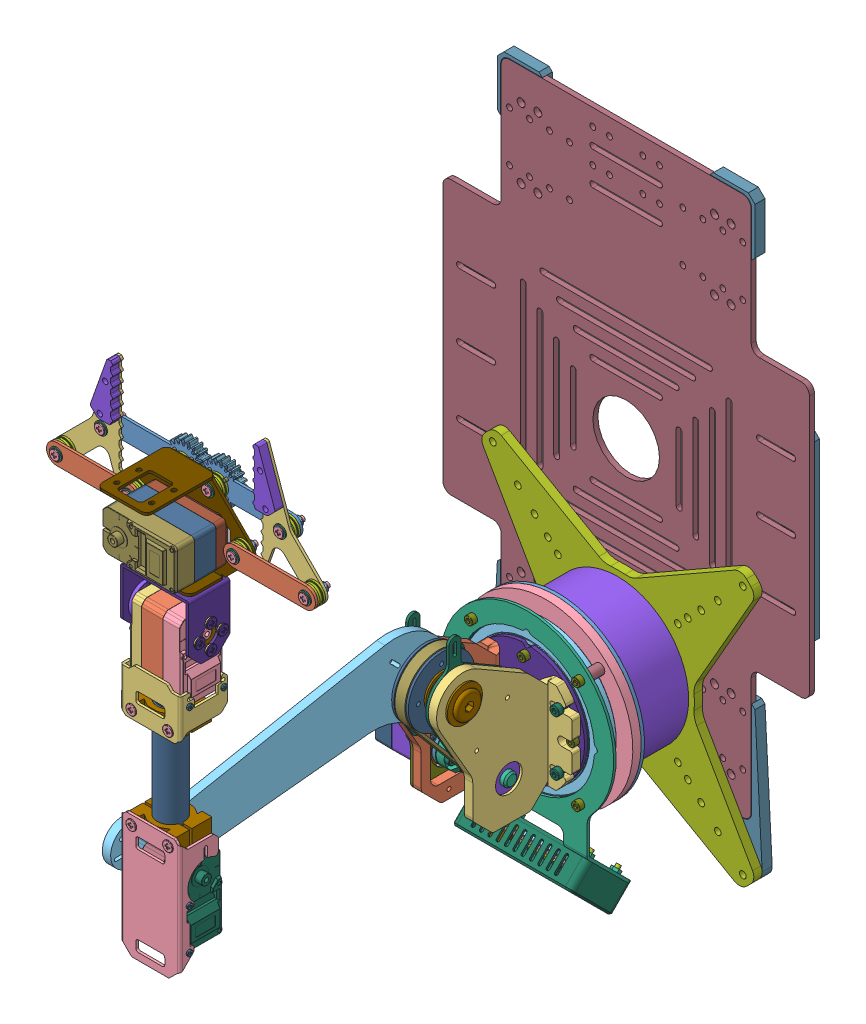
SolidWorks assembly RoArm-M1 STEP, configuration Default. Lengths in mm.
Overall size (220 416.15 679.62).
828 component instances, 340 part files, 15 mates.
Components (placement in the parent):
- RoArm-M1 STEP(2)^RoArm-M1 STEP-1: RoArm-M1 STEP(2)^RoArm-M1 STEP [Default] at origin size (176.32 372.07 316.7) (virtual)
  - 大扭矩云台模块^RoArm-M1 STEP(2)_RoArm-M1 STEP-1: 大扭矩云台模块^RoArm-M1 STEP(2)_RoArm-M1 STEP [Default] at (210 0 0) x (0 1 0) z (0 0 1) size (125.15 106.06 129.64) (virtual)
    - SCS215^大扭矩云台模块_RoArm-M1 STEP(2)_RoArm-M1 STEP-1: SCS215^大扭矩云台模块_RoArm-M1 STEP(2)_RoArm-M1 STEP [Default] at (120 0 0) x (0 1 0) z (1 0 0) size (45.22 37.8 24.72) (virtual)
      - ZK_122^SCS215_大扭矩云台模块_RoArm-M1 STEP(2)_RoArm-M1 STEP-1: ZK_122^SCS215_大扭矩云台模块_RoArm-M1 STEP(2)_RoArm-M1 STEP [Default] at (184.5 34.6 -120) x (-1 0 0) z (0 0 -1) size (45.22 13.9 24.72) (virtual)
      - SG-ZIJI_15^SCS215_大扭矩云台模块_RoArm-M1 STEP(2)_RoArm-M1 STEP-1: SG-ZIJI_15^SCS215_大扭矩云台模块_RoArm-M1 STEP(2)_RoArm-M1 STEP [Default] at (184.5 34.6 -120) x (-1 0 0) z (0 0 -1) size (45 9.77 24.5) (virtual)
      - XG-ZIJI_16^SCS215_大扭矩云台模块_RoArm-M1 STEP(2)_RoArm-M1 STEP-1: XG-ZIJI_16^SCS215_大扭矩云台模块_RoArm-M1 STEP(2)_RoArm-M1 STEP [Default] at (184.5 34.6 -120) x (-1 0 0) z (0 0 -1) size (45.22 14.1 24.72) (virtual)
      - MOTOR-1723_3^SCS215_大扭矩云台模块_RoArm-M1 STEP(2)_RoArm-M1 STEP-1: MOTOR-1723_3^SCS215_大扭矩云台模块_RoArm-M1 STEP(2)_RoArm-M1 STEP [Default] at (184.5 11.75 -118.75) x (0 0 1) z (-1 0 0) size (17.05 30.5 17.05) (virtual)
      - PCB-CHAZUO_92^SCS215_大扭矩云台模块_RoArm-M1 STEP(2)_RoArm-M1 STEP-1: PCB-CHAZUO_92^SCS215_大扭矩云台模块_RoArm-M1 STEP(2)_RoArm-M1 STEP [Default] at (184.5 34.6 -120) x (-1 0 0) z (0 0 -1) size (28.8 7.2 21.1) (virtual)
      - GE_27^SCS215_大扭矩云台模块_RoArm-M1 STEP(2)_RoArm-M1 STEP-1: GE_27^SCS215_大扭矩云台模块_RoArm-M1 STEP(2)_RoArm-M1 STEP [Default] at (210 28.6 -120) x (-1 0 0) z (0 -1 0) size (17.6 17.59 18.3) (virtual)
      - 金属舵盘（驱动）^SCS215_大扭矩云台模块_RoArm-M1 STEP(2)_RoArm-M1 STEP-1: 金属舵盘（驱动）^SCS215_大扭矩云台模块_RoArm-M1 STEP(2)_RoArm-M1 STEP [Default] at (220 17.2 -120) x (-1 0 0) z (0 0 -1) size (19.2 4.5 19.2) (virtual)
    - SCS215_1^大扭矩云台模块_RoArm-M1 STEP(2)_RoArm-M1 STEP-1: SCS215_1^大扭矩云台模块_RoArm-M1 STEP(2)_RoArm-M1 STEP [Default] at (220 0 0) x (-1 0 0) z (0 0 -1) size (45.22 37.8 24.72) (virtual)
      - ZK_122^SCS215_1_大扭矩云台模块_RoArm-M1 STEP(2)_RoArm-M1 STEP-1: ZK_122^SCS215_1_大扭矩云台模块_RoArm-M1 STEP(2)_RoArm-M1 STEP [Default] at (206.3824 235.8615 -88.375) x (-1 0 0) z (0 0 1) size (45.22 13.9 24.72) (virtual)
      - SG-ZIJI_15^SCS215_1_大扭矩云台模块_RoArm-M1 STEP(2)_RoArm-M1 STEP-1: SG-ZIJI_15^SCS215_1_大扭矩云台模块_RoArm-M1 STEP(2)_RoArm-M1 STEP [Default] at (206.3824 235.8615 -88.375) x (-1 0 0) z (0 0 1) size (45 9.77 24.5) (virtual)
      - XG-ZIJI_16^SCS215_1_大扭矩云台模块_RoArm-M1 STEP(2)_RoArm-M1 STEP-1: XG-ZIJI_16^SCS215_1_大扭矩云台模块_RoArm-M1 STEP(2)_RoArm-M1 STEP [Default] at (206.3824 235.8615 -88.375) x (-1 0 0) z (0 0 1) size (45.22 14.1 24.72) (virtual)
      - MOTOR-1723_3^SCS215_1_大扭矩云台模块_RoArm-M1 STEP(2)_RoArm-M1 STEP-1: MOTOR-1723_3^SCS215_1_大扭矩云台模块_RoArm-M1 STEP(2)_RoArm-M1 STEP [Default] at (206.3824 258.7115 -89.625) x (0 0 -1) z (-1 0 0) size (17.05 30.5 17.05) (virtual)
      - PCB-CHAZUO_92^SCS215_1_大扭矩云台模块_RoArm-M1 STEP(2)_RoArm-M1 STEP-1: PCB-CHAZUO_92^SCS215_1_大扭矩云台模块_RoArm-M1 STEP(2)_RoArm-M1 STEP [Default] at (206.3824 235.8615 -88.375) x (-1 0 0) z (0 0 1) size (28.8 7.2 21.1) (virtual)
      - GE_27^SCS215_1_大扭矩云台模块_RoArm-M1 STEP(2)_RoArm-M1 STEP-1: GE_27^SCS215_1_大扭矩云台模块_RoArm-M1 STEP(2)_RoArm-M1 STEP [Default] at (231.8824 241.8615 -88.375) x (-1 0 0) z (0 1 0) size (17.6 17.59 18.3) (virtual)
      - 金属舵盘（驱动）^SCS215_1_大扭矩云台模块_RoArm-M1 STEP(2)_RoArm-M1 STEP-1: 金属舵盘（驱动）^SCS215_1_大扭矩云台模块_RoArm-M1 STEP(2)_RoArm-M1 STEP [Default] at (241.8824 253.2615 -88.375) x (-1 0 0) z (0 0 1) size (19.2 4.5 19.2) (virtual)
    - 校准限位座^大扭矩云台模块_RoArm-M1 STEP(2)_RoArm-M1 STEP-1: 校准限位座^大扭矩云台模块_RoArm-M1 STEP(2)_RoArm-M1 STEP [Default] at (593.7063 198.5385 14.7146) x (1 0 0) z (0 -1 0) size (64.47 46.12 1.5) (virtual)
    - 校准限位座^大扭矩云台模块_RoArm-M1 STEP(2)_RoArm-M1 STEP-2: 校准限位座^大扭矩云台模块_RoArm-M1 STEP(2)_RoArm-M1 STEP [Default] at (593.7063 222.9615 14.7146) x (1 0 0) z (0 -1 0) size (64.47 46.12 1.5) (virtual)
    - 舵机支架^大扭矩云台模块_RoArm-M1 STEP(2)_RoArm-M1 STEP-1: 舵机支架^大扭矩云台模块_RoArm-M1 STEP(2)_RoArm-M1 STEP [Default] at (563.2369 229.4615 83.2872) x (1 0 0) z (0 -1 0) size (70.99 43.89 1.5) (virtual)
    - 中心旋转上面^大扭矩云台模块_RoArm-M1 STEP(2)_RoArm-M1 STEP-1: 中心旋转上面^大扭矩云台模块_RoArm-M1 STEP(2)_RoArm-M1 STEP [Default] at (-103.1005 341.7844 58) x (-1 0 0) z (0 0 1) size (69.72 70 2) (virtual)
    - 中心旋转下面^大扭矩云台模块_RoArm-M1 STEP(2)_RoArm-M1 STEP-1: 中心旋转下面^大扭矩云台模块_RoArm-M1 STEP(2)_RoArm-M1 STEP [Default] at (-99.0694 230.427 46) x (-1 0 0) z (0 0 1) size (70 70 2) (virtual)
    - 中心舵机支架^大扭矩云台模块_RoArm-M1 STEP(2)_RoArm-M1 STEP-1: 中心舵机支架^大扭矩云台模块_RoArm-M1 STEP(2)_RoArm-M1 STEP [Default] at (-104.8058 305.9776 41) x (0 1 0) z (0 0 1) size (104 104 2) (virtual)
    - 云台驱动侧^大扭矩云台模块_RoArm-M1 STEP(2)_RoArm-M1 STEP-1: 云台驱动侧^大扭矩云台模块_RoArm-M1 STEP(2)_RoArm-M1 STEP [Default] at (-313.1456 227.9615 126.4297) x (1 0 0) z (0 -1 0) size (92.37 71.79 19.59) (virtual)
    - 云台从动侧^大扭矩云台模块_RoArm-M1 STEP(2)_RoArm-M1 STEP-1: 云台从动侧^大扭矩云台模块_RoArm-M1 STEP(2)_RoArm-M1 STEP [Default] at (-304.3961 197.0385 -7.6382) x (1 0 0) z (0 -1 0) size (92.37 71.79 19.59) (virtual)
    - 结构底座^大扭矩云台模块_RoArm-M1 STEP(2)_RoArm-M1 STEP-1: 结构底座^大扭矩云台模块_RoArm-M1 STEP(2)_RoArm-M1 STEP [Default] at (273.7799 14.8085 43) x (-1 0 0) z (0 0 1) size (104 104 5) (virtual)
    - 深沟球轴承 6813RS^大扭矩云台模块_RoArm-M1 STEP(2)_RoArm-M1 STEP-1: 深沟球轴承 6813RS^大扭矩云台模块_RoArm-M1 STEP(2)_RoArm-M1 STEP [Default] at (0 210 48) x (-1 0 0) z (0 0 1) size (85 85 10) (virtual)
    - 舵机法兰盘^大扭矩云台模块_RoArm-M1 STEP(2)_RoArm-M1 STEP-1: 舵机法兰盘^大扭矩云台模块_RoArm-M1 STEP(2)_RoArm-M1 STEP [Default] at (-11.8824 226.2615 88.375) x (-1 0 0) z (0 -1 0) size (18.8 18.8 36.24) (virtual)
    - GT2 20T5B_dz2020^大扭矩云台模块_RoArm-M1 STEP(2)_RoArm-M1 STEP-1: GT2 20T5B_dz2020^大扭矩云台模块_RoArm-M1 STEP(2)_RoArm-M1 STEP [Default] at (-11.8824 206.2615 88.375) x (-1 0 0) z (0 1 0) size (15.01 15.01 16) (virtual)
    - 法兰轴承 F688ZZ^大扭矩云台模块_RoArm-M1 STEP(2)_RoArm-M1 STEP-1: 法兰轴承 F688ZZ^大扭矩云台模块_RoArm-M1 STEP(2)_RoArm-M1 STEP [Default] at (-11.8824 198.4615 88.375) x (-1 0 0) z (0 -1 0) size (18 18 5) (virtual)
    - 法兰轴承 F6800ZZ^大扭矩云台模块_RoArm-M1 STEP(2)_RoArm-M1 STEP-1: 法兰轴承 F6800ZZ^大扭矩云台模块_RoArm-M1 STEP(2)_RoArm-M1 STEP [Default] at (41.0513 191.0385 115.7401) x (-1 0 0) z (0 1 0) size (21 21 5) (virtual)
    - 法兰轴承 F6800ZZ^大扭矩云台模块_RoArm-M1 STEP(2)_RoArm-M1 STEP-2: 法兰轴承 F6800ZZ^大扭矩云台模块_RoArm-M1 STEP(2)_RoArm-M1 STEP [Default] at (41.0513 228.9615 115.7401) x (1 0 0) z (0 -1 0) size (21 21 5) (virtual)
    - 定制同步轮 2GT 60T 平面孔^大扭矩云台模块_RoArm-M1 STEP(2)_RoArm-M1 STEP-1: 定制同步轮 2GT 60T 平面孔^大扭矩云台模块_RoArm-M1 STEP(2)_RoArm-M1 STEP [Default] at (-237.2373 206.3615 -141.3792) x (-1 0 0) z (0 1 0) size (40 40 10) (virtual)
    - 法兰轴承 F6800ZZ^大扭矩云台模块_RoArm-M1 STEP(2)_RoArm-M1 STEP-3: 法兰轴承 F6800ZZ^大扭矩云台模块_RoArm-M1 STEP(2)_RoArm-M1 STEP [Default] at (41.0513 215.9615 115.7401) x (1 0 0) z (0 -1 0) size (21 21 5) (virtual)
    - 法兰轴承 F6800ZZ^大扭矩云台模块_RoArm-M1 STEP(2)_RoArm-M1 STEP-4: 法兰轴承 F6800ZZ^大扭矩云台模块_RoArm-M1 STEP(2)_RoArm-M1 STEP [Default] at (41.0513 203.9615 115.7401) x (-1 0 0) z (0 1 0) size (21 21 5) (virtual)
    - 平面轴承 F10-18M^大扭矩云台模块_RoArm-M1 STEP(2)_RoArm-M1 STEP-1: 平面轴承 F10-18M^大扭矩云台模块_RoArm-M1 STEP(2)_RoArm-M1 STEP [Default] at (41.0513 221.4615 115.7401) x (-1 0 0) z (0 -1 0) size (18 18 5.5) (virtual)
    - 平面轴承 F10-18M^大扭矩云台模块_RoArm-M1 STEP(2)_RoArm-M1 STEP-2: 平面轴承 F10-18M^大扭矩云台模块_RoArm-M1 STEP(2)_RoArm-M1 STEP [Default] at (41.0513 203.9615 115.7401) x (-1 0 0) z (0 -1 0) size (18 18 5.5) (virtual)
    - 200mm 同步带^大扭矩云台模块_RoArm-M1 STEP(2)_RoArm-M1 STEP-1: 200mm 同步带^大扭矩云台模块_RoArm-M1 STEP(2)_RoArm-M1 STEP [Default] at (-3454.3519 217.7615 -3952.2418) x (1 0 0) z (0 -1 0) size (80.23 54.67 6) (virtual)
  - SCS215_2^RoArm-M1 STEP(2)_RoArm-M1 STEP-1: SCS215_2^RoArm-M1 STEP(2)_RoArm-M1 STEP [Default] at (0 -140 0) x (0 -1 0) z (0 0 1) size (45.22 37.8 24.72) (virtual)
    - ZK_122^SCS215_2_RoArm-M1 STEP(2)_RoArm-M1 STEP-1: ZK_122^SCS215_2_RoArm-M1 STEP(2)_RoArm-M1 STEP [Default] at (-155.5513 4.6385 284.598) x (1 0 0) z (0 0 -1) size (45.22 13.9 24.72) (virtual)
    - SG-ZIJI_15^SCS215_2_RoArm-M1 STEP(2)_RoArm-M1 STEP-1: SG-ZIJI_15^SCS215_2_RoArm-M1 STEP(2)_RoArm-M1 STEP [Default] at (-155.5513 4.6385 284.598) x (1 0 0) z (0 0 -1) size (45 9.77 24.5) (virtual)
    - XG-ZIJI_16^SCS215_2_RoArm-M1 STEP(2)_RoArm-M1 STEP-1: XG-ZIJI_16^SCS215_2_RoArm-M1 STEP(2)_RoArm-M1 STEP [Default] at (-155.5513 4.6385 284.598) x (1 0 0) z (0 0 -1) size (45.22 14.1 24.72) (virtual)
    - MOTOR-1723_3^SCS215_2_RoArm-M1 STEP(2)_RoArm-M1 STEP-1: MOTOR-1723_3^SCS215_2_RoArm-M1 STEP(2)_RoArm-M1 STEP [Default] at (-155.5513 27.4885 285.848) x (0 0 1) z (1 0 0) size (17.05 30.5 17.05) (virtual)
    - PCB-CHAZUO_92^SCS215_2_RoArm-M1 STEP(2)_RoArm-M1 STEP-1: PCB-CHAZUO_92^SCS215_2_RoArm-M1 STEP(2)_RoArm-M1 STEP [Default] at (-155.5513 4.6385 284.598) x (1 0 0) z (0 0 -1) size (28.8 7.2 21.1) (virtual)
    - GE_27^SCS215_2_RoArm-M1 STEP(2)_RoArm-M1 STEP-1: GE_27^SCS215_2_RoArm-M1 STEP(2)_RoArm-M1 STEP [Default] at (-181.0513 10.6385 284.598) x (1 0 0) z (0 1 0) size (17.6 17.59 18.3) (virtual)
    - 金属舵盘（驱动）^SCS215_2_RoArm-M1 STEP(2)_RoArm-M1 STEP-1: 金属舵盘（驱动）^SCS215_2_RoArm-M1 STEP(2)_RoArm-M1 STEP [Default] at (-191.0513 22.0385 284.598) x (1 0 0) z (0 0 -1) size (19.2 4.5 19.2) (virtual)
  - SCS215_3^RoArm-M1 STEP(2)_RoArm-M1 STEP-1: SCS215_3^RoArm-M1 STEP(2)_RoArm-M1 STEP [Default] at (110 -140 0) x (0 -1 0) z (0 0 1) size (45.22 37.8 24.72) (virtual)
    - ZK_122^SCS215_3_RoArm-M1 STEP(2)_RoArm-M1 STEP-1: ZK_122^SCS215_3_RoArm-M1 STEP(2)_RoArm-M1 STEP [Default] at (-283.4747 -105.0615 284.598) x (1 0 0) z (0 0 -1) size (45.22 13.9 24.72) (virtual)
    - SG-ZIJI_15^SCS215_3_RoArm-M1 STEP(2)_RoArm-M1 STEP-1: SG-ZIJI_15^SCS215_3_RoArm-M1 STEP(2)_RoArm-M1 STEP [Default] at (-283.4747 -105.0615 284.598) x (1 0 0) z (0 0 -1) size (45 9.77 24.5) (virtual)
    - XG-ZIJI_16^SCS215_3_RoArm-M1 STEP(2)_RoArm-M1 STEP-1: XG-ZIJI_16^SCS215_3_RoArm-M1 STEP(2)_RoArm-M1 STEP [Default] at (-283.4747 -105.0615 284.598) x (1 0 0) z (0 0 -1) size (45.22 14.1 24.72) (virtual)
    - MOTOR-1723_3^SCS215_3_RoArm-M1 STEP(2)_RoArm-M1 STEP-1: MOTOR-1723_3^SCS215_3_RoArm-M1 STEP(2)_RoArm-M1 STEP [Default] at (-283.4747 -82.2115 285.848) x (0 0 1) z (1 0 0) size (17.05 30.5 17.05) (virtual)
    - PCB-CHAZUO_92^SCS215_3_RoArm-M1 STEP(2)_RoArm-M1 STEP-1: PCB-CHAZUO_92^SCS215_3_RoArm-M1 STEP(2)_RoArm-M1 STEP [Default] at (-283.4747 -105.0615 284.598) x (1 0 0) z (0 0 -1) size (28.8 7.2 21.1) (virtual)
    - GE_27^SCS215_3_RoArm-M1 STEP(2)_RoArm-M1 STEP-1: GE_27^SCS215_3_RoArm-M1 STEP(2)_RoArm-M1 STEP [Default] at (-308.9747 -99.0615 284.598) x (1 0 0) z (0 1 0) size (17.6 17.59 18.3) (virtual)
    - 金属舵盘（驱动）^SCS215_3_RoArm-M1 STEP(2)_RoArm-M1 STEP-1: 金属舵盘（驱动）^SCS215_3_RoArm-M1 STEP(2)_RoArm-M1 STEP [Default] at (-318.9747 -87.6615 284.598) x (1 0 0) z (0 0 -1) size (19.2 4.5 19.2) (virtual)
    - 金属舵盘（从动）^SCS215_3_RoArm-M1 STEP(2)_RoArm-M1 STEP-1: 金属舵盘（从动）^SCS215_3_RoArm-M1 STEP(2)_RoArm-M1 STEP [Default] at (-298.9747 -55.6115 284.598) x (-1 0 0) z (0 0 -1) size (19.2 3.35 19.2) (virtual)
  - 铝合金夹头^RoArm-M1 STEP(2)_RoArm-M1 STEP-1: 铝合金夹头^RoArm-M1 STEP(2)_RoArm-M1 STEP [Default] at (0 -300 0) size (161.4 120.87 54.76) (virtual)
    - SCS215_4^铝合金夹头_RoArm-M1 STEP(2)_RoArm-M1 STEP-1: SCS215_4^铝合金夹头_RoArm-M1 STEP(2)_RoArm-M1 STEP [Default] at (0 -80 0) x (-1 0 0) z (0 -1 0) size (45.22 37.8 24.72) (virtual)
      - ZK_122^SCS215_4_铝合金夹头_RoArm-M1 STEP(2)_RoArm-M1 STEP-1: ZK_122^SCS215_4_铝合金夹头_RoArm-M1 STEP(2)_RoArm-M1 STEP [Default] at (-26.9885 -281.5404 -594.0059) x (-1 0 0) z (0 0 -1) size (45.22 13.9 24.72) (virtual)
      - SG-ZIJI_15^SCS215_4_铝合金夹头_RoArm-M1 STEP(2)_RoArm-M1 STEP-1: SG-ZIJI_15^SCS215_4_铝合金夹头_RoArm-M1 STEP(2)_RoArm-M1 STEP [Default] at (-26.9885 -281.5404 -594.0059) x (-1 0 0) z (0 0 -1) size (45 9.77 24.5) (virtual)
      - XG-ZIJI_16^SCS215_4_铝合金夹头_RoArm-M1 STEP(2)_RoArm-M1 STEP-1: XG-ZIJI_16^SCS215_4_铝合金夹头_RoArm-M1 STEP(2)_RoArm-M1 STEP [Default] at (-26.9885 -281.5404 -594.0059) x (-1 0 0) z (0 0 -1) size (45.22 14.1 24.72) (virtual)
      - MOTOR-1723_3^SCS215_4_铝合金夹头_RoArm-M1 STEP(2)_RoArm-M1 STEP-1: MOTOR-1723_3^SCS215_4_铝合金夹头_RoArm-M1 STEP(2)_RoArm-M1 STEP [Default] at (-26.9885 -304.3904 -592.7559) x (0 0 1) z (-1 0 0) size (17.05 30.5 17.05) (virtual)
      - PCB-CHAZUO_92^SCS215_4_铝合金夹头_RoArm-M1 STEP(2)_RoArm-M1 STEP-1: PCB-CHAZUO_92^SCS215_4_铝合金夹头_RoArm-M1 STEP(2)_RoArm-M1 STEP [Default] at (-26.9885 -281.5404 -594.0059) x (-1 0 0) z (0 0 -1) size (28.8 7.2 21.1) (virtual)
      - GE_27^SCS215_4_铝合金夹头_RoArm-M1 STEP(2)_RoArm-M1 STEP-1: GE_27^SCS215_4_铝合金夹头_RoArm-M1 STEP(2)_RoArm-M1 STEP [Default] at (-1.4885 -287.5404 -594.0059) x (-1 0 0) z (0 -1 0) size (17.6 17.59 18.3) (virtual)
      - 金属舵盘（驱动）^SCS215_4_铝合金夹头_RoArm-M1 STEP(2)_RoArm-M1 STEP-1: 金属舵盘（驱动）^SCS215_4_铝合金夹头_RoArm-M1 STEP(2)_RoArm-M1 STEP [Default] at (8.5115 -298.9404 -594.0059) x (-1 0 0) z (0 0 -1) size (19.2 4.5 19.2) (virtual)
    - Theta舵机支架^铝合金夹头_RoArm-M1 STEP(2)_RoArm-M1 STEP-1: Theta舵机支架^铝合金夹头_RoArm-M1 STEP(2)_RoArm-M1 STEP [Default] at (-169.3904 490.9147 215.0784) x (-1 0 0) z (0 1 0) size (41.02 24.76 35.78) (virtual)
    - 夹头底座^铝合金夹头_RoArm-M1 STEP(2)_RoArm-M1 STEP-1: 夹头底座^铝合金夹头_RoArm-M1 STEP(2)_RoArm-M1 STEP [Default] at (186.1989 491.5088 275.1404) x (1 0 0) z (0 0 -1) size (75 52.69 43.11) (virtual)
    - 齿轮臂^铝合金夹头_RoArm-M1 STEP(2)_RoArm-M1 STEP-1: 齿轮臂^铝合金夹头_RoArm-M1 STEP(2)_RoArm-M1 STEP [Default] at (142.6435 364.0906 267.6404) x (0 -1 0) z (0 0 1) size (22.92 60.69 1.5) (virtual)
    - 齿轮臂^铝合金夹头_RoArm-M1 STEP(2)_RoArm-M1 STEP-2: 齿轮臂^铝合金夹头_RoArm-M1 STEP(2)_RoArm-M1 STEP [Default] at (-114.6664 705.7304 267.6404) x (0 1 0) z (0 0 1) size (22.92 60.69 1.5) (virtual)
    - 夹头从动臂^铝合金夹头_RoArm-M1 STEP(2)_RoArm-M1 STEP-1: 夹头从动臂^铝合金夹头_RoArm-M1 STEP(2)_RoArm-M1 STEP [Default] at (-114.3325 284.3731 279.6404) x (-1 0 0) z (0 0 1) size (55.2 12 1.5) (virtual)
    - 夹头从动臂^铝合金夹头_RoArm-M1 STEP(2)_RoArm-M1 STEP-2: 夹头从动臂^铝合金夹头_RoArm-M1 STEP(2)_RoArm-M1 STEP [Default] at (-220.5325 284.3731 279.6404) x (-1 0 0) z (0 0 1) size (55.2 12 1.5) (virtual)
    - 夹头末端^铝合金夹头_RoArm-M1 STEP(2)_RoArm-M1 STEP-1: 夹头末端^铝合金夹头_RoArm-M1 STEP(2)_RoArm-M1 STEP [Default] at (127.1252 235.8839 275.1404) x (1 0 0) z (0 0 -1) size (38.61 69.6 1.5) (virtual)
    - 夹头末端^铝合金夹头_RoArm-M1 STEP(2)_RoArm-M1 STEP-2: 夹头末端^铝合金夹头_RoArm-M1 STEP(2)_RoArm-M1 STEP [Default] at (-99.1481 235.8839 273.6404) x (-1 0 0) z (0 0 1) size (38.61 69.6 1.5) (virtual)
    - 舵机驱动加强齿^铝合金夹头_RoArm-M1 STEP(2)_RoArm-M1 STEP-1: 舵机驱动加强齿^铝合金夹头_RoArm-M1 STEP(2)_RoArm-M1 STEP [Default] at (37.7378 637.1469 266.9404) x (-0.707107 -0.707107 0) z (0 0 1) size (22.92 22.98 5) (virtual)
    - 从动加强齿^铝合金夹头_RoArm-M1 STEP(2)_RoArm-M1 STEP-1: 从动加强齿^铝合金夹头_RoArm-M1 STEP(2)_RoArm-M1 STEP [Default] at (33.5278 422.432 262.6404) x (0 1 0) z (0 0 1) size (22.92 22.98 5) (virtual)
    - 从动加强齿^铝合金夹头_RoArm-M1 STEP(2)_RoArm-M1 STEP-2: 从动加强齿^铝合金夹头_RoArm-M1 STEP(2)_RoArm-M1 STEP [Default] at (-5.5507 647.389 262.6404) x (0 -1 0) z (0 0 1) size (22.92 22.98 5) (virtual)
    - MF63ZZ^铝合金夹头_RoArm-M1 STEP(2)_RoArm-M1 STEP-1: MF63ZZ^铝合金夹头_RoArm-M1 STEP(2)_RoArm-M1 STEP [Default] at (24.4885 534.9105 275.7404) x (1 0 0) z (0 0 -1) size (7.2 7.2 2.5) (virtual)
    - MF63ZZ^铝合金夹头_RoArm-M1 STEP(2)_RoArm-M1 STEP-2: MF63ZZ^铝合金夹头_RoArm-M1 STEP(2)_RoArm-M1 STEP [Default] at (3.4885 534.9105 275.7404) x (1 0 0) z (0 0 -1) size (7.2 7.2 2.5) (virtual)
    - MF63ZZ^铝合金夹头_RoArm-M1 STEP(2)_RoArm-M1 STEP-3: MF63ZZ^铝合金夹头_RoArm-M1 STEP(2)_RoArm-M1 STEP [Default] at (45.4885 513.9105 273.0404) x (-1 0 0) z (0 0 1) size (7.2 7.2 2.5) (virtual)
    - MF63ZZ^铝合金夹头_RoArm-M1 STEP(2)_RoArm-M1 STEP-4: MF63ZZ^铝合金夹头_RoArm-M1 STEP(2)_RoArm-M1 STEP [Default] at (-17.5115 513.9105 273.0404) x (-1 0 0) z (0 0 1) size (7.2 7.2 2.5) (virtual)
    - 平面轴承 F6-12^铝合金夹头_RoArm-M1 STEP(2)_RoArm-M1 STEP-1: 平面轴承 F6-12^铝合金夹头_RoArm-M1 STEP(2)_RoArm-M1 STEP [Default] at (24.4885 534.9105 269.1404) x (-1 0 0) z (0 0 1) size (12 12 4.5) (virtual)
    - 平面轴承 F6-12^铝合金夹头_RoArm-M1 STEP(2)_RoArm-M1 STEP-2: 平面轴承 F6-12^铝合金夹头_RoArm-M1 STEP(2)_RoArm-M1 STEP [Default] at (3.4885 534.9105 269.1404) x (-1 0 0) z (0 0 1) size (12 12 4.5) (virtual)
    - 平面轴承 F6-12^铝合金夹头_RoArm-M1 STEP(2)_RoArm-M1 STEP-3: 平面轴承 F6-12^铝合金夹头_RoArm-M1 STEP(2)_RoArm-M1 STEP [Default] at (45.4885 513.9105 275.1404) x (-1 0 0) z (0 0 1) size (12 12 4.5) (virtual)
    - 平面轴承 F6-12^铝合金夹头_RoArm-M1 STEP(2)_RoArm-M1 STEP-4: 平面轴承 F6-12^铝合金夹头_RoArm-M1 STEP(2)_RoArm-M1 STEP [Default] at (-17.5115 513.9105 275.1404) x (-1 0 0) z (0 0 1) size (12 12 4.5) (virtual)
    - MF63ZZ^铝合金夹头_RoArm-M1 STEP(2)_RoArm-M1 STEP-5: MF63ZZ^铝合金夹头_RoArm-M1 STEP(2)_RoArm-M1 STEP [Default] at (-60.7115 513.9105 281.7404) x (1 0 0) z (0 0 -1) size (7.2 7.2 2.5) (virtual)
    - MF63ZZ^铝合金夹头_RoArm-M1 STEP(2)_RoArm-M1 STEP-6: MF63ZZ^铝合金夹头_RoArm-M1 STEP(2)_RoArm-M1 STEP [Default] at (-17.5115 513.9105 281.7404) x (1 0 0) z (0 0 -1) size (7.2 7.2 2.5) (virtual)
    - MF63ZZ^铝合金夹头_RoArm-M1 STEP(2)_RoArm-M1 STEP-7: MF63ZZ^铝合金夹头_RoArm-M1 STEP(2)_RoArm-M1 STEP [Default] at (45.4885 513.9105 281.7404) x (1 0 0) z (0 0 -1) size (7.2 7.2 2.5) (virtual)
    - MF63ZZ^铝合金夹头_RoArm-M1 STEP(2)_RoArm-M1 STEP-8: MF63ZZ^铝合金夹头_RoArm-M1 STEP(2)_RoArm-M1 STEP [Default] at (88.6885 513.9105 281.7404) x (1 0 0) z (0 0 -1) size (7.2 7.2 2.5) (virtual)
    - MF63ZZ^铝合金夹头_RoArm-M1 STEP(2)_RoArm-M1 STEP-9: MF63ZZ^铝合金夹头_RoArm-M1 STEP(2)_RoArm-M1 STEP [Default] at (24.4885 534.9105 267.0404) x (0 1 0) z (0 0 1) size (7.2 7.2 2.5) (virtual)
    - MF63ZZ^铝合金夹头_RoArm-M1 STEP(2)_RoArm-M1 STEP-10: MF63ZZ^铝合金夹头_RoArm-M1 STEP(2)_RoArm-M1 STEP [Default] at (3.4885 534.9105 267.0404) x (0 -1 0) z (0 0 1) size (7.2 7.2 2.5) (virtual)
    - MF63ZZ^铝合金夹头_RoArm-M1 STEP(2)_RoArm-M1 STEP-11: MF63ZZ^铝合金夹头_RoArm-M1 STEP(2)_RoArm-M1 STEP [Default] at (-39.7115 534.9105 267.0404) x (0 -1 0) z (0 0 1) size (7.2 7.2 2.5) (virtual)
    - MF63ZZ^铝合金夹头_RoArm-M1 STEP(2)_RoArm-M1 STEP-12: MF63ZZ^铝合金夹头_RoArm-M1 STEP(2)_RoArm-M1 STEP [Default] at (67.6885 534.9105 267.0404) x (0 1 0) z (0 0 1) size (7.2 7.2 2.5) (virtual)
    - 平面轴承 F6-12^铝合金夹头_RoArm-M1 STEP(2)_RoArm-M1 STEP-5: 平面轴承 F6-12^铝合金夹头_RoArm-M1 STEP(2)_RoArm-M1 STEP [Default] at (-39.7115 534.9105 269.1404) x (0 -1 0) z (0 0 1) size (12 12 4.5) (virtual)
    - 平面轴承 F6-12^铝合金夹头_RoArm-M1 STEP(2)_RoArm-M1 STEP-6: 平面轴承 F6-12^铝合金夹头_RoArm-M1 STEP(2)_RoArm-M1 STEP [Default] at (67.6885 534.9105 269.1404) x (0 1 0) z (0 0 1) size (12 12 4.5) (virtual)
    - 舵机驱动加强齿^铝合金夹头_RoArm-M1 STEP(2)_RoArm-M1 STEP-2: 舵机驱动加强齿^铝合金夹头_RoArm-M1 STEP(2)_RoArm-M1 STEP [Default] at (37.7378 637.1469 261.9404) x (-0.707107 -0.707107 0) z (0 0 1) size (22.92 22.98 5) (virtual)
    - MF63ZZ^铝合金夹头_RoArm-M1 STEP(2)_RoArm-M1 STEP-13: MF63ZZ^铝合金夹头_RoArm-M1 STEP(2)_RoArm-M1 STEP [Default] at (88.6885 513.9105 273.0404) x (-1 0 0) z (0 0 1) size (7.2 7.2 2.5) (virtual)
    - MF63ZZ^铝合金夹头_RoArm-M1 STEP(2)_RoArm-M1 STEP-14: MF63ZZ^铝合金夹头_RoArm-M1 STEP(2)_RoArm-M1 STEP [Default] at (67.6885 534.9105 275.7404) x (1 0 0) z (0 0 -1) size (7.2 7.2 2.5) (virtual)
    - MF63ZZ^铝合金夹头_RoArm-M1 STEP(2)_RoArm-M1 STEP-15: MF63ZZ^铝合金夹头_RoArm-M1 STEP(2)_RoArm-M1 STEP [Default] at (-60.7115 513.9105 273.0404) x (-1 0 0) z (0 0 1) size (7.2 7.2 2.5) (virtual)
    - MF63ZZ^铝合金夹头_RoArm-M1 STEP(2)_RoArm-M1 STEP-16: MF63ZZ^铝合金夹头_RoArm-M1 STEP(2)_RoArm-M1 STEP [Default] at (-39.7115 534.9105 275.7404) x (1 0 0) z (0 0 -1) size (7.2 7.2 2.5) (virtual)
    - 平面轴承 F6-12^铝合金夹头_RoArm-M1 STEP(2)_RoArm-M1 STEP-7: 平面轴承 F6-12^铝合金夹头_RoArm-M1 STEP(2)_RoArm-M1 STEP [Default] at (88.6885 513.9105 275.1404) x (-1 0 0) z (0 0 1) size (12 12 4.5) (virtual)
    - 平面轴承 F6-12^铝合金夹头_RoArm-M1 STEP(2)_RoArm-M1 STEP-8: 平面轴承 F6-12^铝合金夹头_RoArm-M1 STEP(2)_RoArm-M1 STEP [Default] at (-60.7115 513.9105 275.1404) x (-1 0 0) z (0 0 1) size (12 12 4.5) (virtual)
    - 夹头末端加强^铝合金夹头_RoArm-M1 STEP(2)_RoArm-M1 STEP-1: 夹头末端加强^铝合金夹头_RoArm-M1 STEP(2)_RoArm-M1 STEP [Default] at (177.6748 496.9439 275.1404) x (-1 0 0) z (0 0 1) size (13.34 33.6 5) (virtual)
    - 夹头末端加强^铝合金夹头_RoArm-M1 STEP(2)_RoArm-M1 STEP-2: 夹头末端加强^铝合金夹头_RoArm-M1 STEP(2)_RoArm-M1 STEP [Default] at (-149.6977 496.9439 280.1404) x (1 0 0) z (0 0 -1) size (13.34 33.6 5) (virtual)
  - Servo Driver with ESP32^RoArm-M1 STEP(2)_RoArm-M1 STEP-1: Servo Driver with ESP32^RoArm-M1 STEP(2)_RoArm-M1 STEP [Default] at (-32.5 -89.0448 39.0323) x (1 0 0) z (0 -0.707107 0.707107) size (65.89 30.51 11.2) (virtual)
    - C23^Servo Driver with ESP32_RoArm-M1 STEP(2)_RoArm-M1 STEP-1: C23^Servo Driver with ESP32_RoArm-M1 STEP(2)_RoArm-M1 STEP [Default] at origin size (1.51 3.44 0.46) (virtual)
      - 490328720^C23_Servo Driver with ESP32_RoArm-M1 STEP(2)_RoArm-M1 STEP-1: 490328720^C23_Servo Driver with ESP32_RoArm-M1 STEP(2)_RoArm-M1 STEP [Default] at (10.8577 24.6493 -0.8715) size (1.51 0.28 0.46) (virtual)
        - Extruded^490328720_C23_Servo Driver with ESP32_RoArm-M1 STEP(2)_RoArm-M1 STEP-1: Extruded^490328720_C23_Servo Driver with ESP32_RoArm-M1 STEP(2)_RoArm-M1 STEP [Default] at origin size (1.51 0.28 0.46) (virtual)
      - 490328720_1^C23_Servo Driver with ESP32_RoArm-M1 STEP(2)_RoArm-M1 STEP-1: 490328720_1^C23_Servo Driver with ESP32_RoArm-M1 STEP(2)_RoArm-M1 STEP [Default] at (10.8576 27.8117 -0.8715) size (1.51 0.28 0.46) (virtual)
        - Extruded^490328720_1_C23_Servo Driver with ESP32_RoArm-M1 STEP(2)_RoArm-M1 STEP-1: Extruded^490328720_1_C23_Servo Driver with ESP32_RoArm-M1 STEP(2)_RoArm-M1 STEP [Default] at origin size (1.51 0.28 0.46) (virtual)
      - 731907408^C23_Servo Driver with ESP32_RoArm-M1 STEP(2)_RoArm-M1 STEP-1: 731907408^C23_Servo Driver with ESP32_RoArm-M1 STEP(2)_RoArm-M1 STEP [Default] at (10.8497 26.2242 -0.8615) size (1.38 3.05 0.42) (virtual)
        - Extruded (1)^731907408_C23_Servo Driver with ESP32_RoArm-M1 STEP(2)_RoArm-M1 STEP-1: Extruded (1)^731907408_C23_Servo Driver with ESP32_RoArm-M1 STEP(2)_RoArm-M1 STEP [Default] at origin size (1.38 3.05 0.42) (virtual)
    - C22^Servo Driver with ESP32_RoArm-M1 STEP(2)_RoArm-M1 STEP-1: C22^Servo Driver with ESP32_RoArm-M1 STEP(2)_RoArm-M1 STEP [Default] at origin size (0.85 1.65 0.46) (virtual)
      - 490325008^C22_Servo Driver with ESP32_RoArm-M1 STEP(2)_RoArm-M1 STEP-1: 490325008^C22_Servo Driver with ESP32_RoArm-M1 STEP(2)_RoArm-M1 STEP [Default] at (8.9576 25.7142 -0.8715) size (0.85 0.28 0.46) (virtual)
        - Extruded (2)^490325008_C22_Servo Driver with ESP32_RoArm-M1 STEP(2)_RoArm-M1 STEP-1: Extruded (2)^490325008_C22_Servo Driver with ESP32_RoArm-M1 STEP(2)_RoArm-M1 STEP [Default] at origin size (0.85 0.28 0.46) (virtual)
      - 490325008_1^C22_Servo Driver with ESP32_RoArm-M1 STEP(2)_RoArm-M1 STEP-1: 490325008_1^C22_Servo Driver with ESP32_RoArm-M1 STEP(2)_RoArm-M1 STEP [Default] at (8.9576 27.0857 -0.8715) size (0.85 0.28 0.46) (virtual)
        - Extruded (2)^490325008_1_C22_Servo Driver with ESP32_RoArm-M1 STEP(2)_RoArm-M1 STEP-1: Extruded (2)^490325008_1_C22_Servo Driver with ESP32_RoArm-M1 STEP(2)_RoArm-M1 STEP [Default] at origin size (0.85 0.28 0.46) (virtual)
      - 490325136^C22_Servo Driver with ESP32_RoArm-M1 STEP(2)_RoArm-M1 STEP-1: 490325136^C22_Servo Driver with ESP32_RoArm-M1 STEP(2)_RoArm-M1 STEP [Default] at (8.9576 26.3999 -0.8615) size (0.8 1.5 0.42) (virtual)
        - Extruded (3)^490325136_C22_Servo Driver with ESP32_RoArm-M1 STEP(2)_RoArm-M1 STEP-1: Extruded (3)^490325136_C22_Servo Driver with ESP32_RoArm-M1 STEP(2)_RoArm-M1 STEP [Default] at origin size (0.8 1.5 0.42) (virtual)
    - U5^Servo Driver with ESP32_RoArm-M1 STEP(2)_RoArm-M1 STEP-1: U5^Servo Driver with ESP32_RoArm-M1 STEP(2)_RoArm-M1 STEP [Default] at origin size (1.81 1.7 0.55) (virtual)
      - 731907024^U5_Servo Driver with ESP32_RoArm-M1 STEP(2)_RoArm-M1 STEP-1: 731907024^U5_Servo Driver with ESP32_RoArm-M1 STEP(2)_RoArm-M1 STEP [Default] at (16.3421 9.6502 0.045) size (1.3 1.7 0.5) (virtual)
        - Extruded (4)^731907024_U5_Servo Driver with ESP32_RoArm-M1 STEP(2)_RoArm-M1 STEP-1: Extruded (4)^731907024_U5_Servo Driver with ESP32_RoArm-M1 STEP(2)_RoArm-M1 STEP [Default] at origin size (1.3 1.7 0.5) (virtual)
      - 490332176^U5_Servo Driver with ESP32_RoArm-M1 STEP(2)_RoArm-M1 STEP-1: 490332176^U5_Servo Driver with ESP32_RoArm-M1 STEP(2)_RoArm-M1 STEP [Default] at (17.0443 9.1502 0) size (0.4 0.23 0.16) (virtual)
        - Extruded (5)^490332176_U5_Servo Driver with ESP32_RoArm-M1 STEP(2)_RoArm-M1 STEP-1: Extruded (5)^490332176_U5_Servo Driver with ESP32_RoArm-M1 STEP(2)_RoArm-M1 STEP [Default] at origin size (0.4 0.23 0.16) (virtual)
      - 490332176_1^U5_Servo Driver with ESP32_RoArm-M1 STEP(2)_RoArm-M1 STEP-1: 490332176_1^U5_Servo Driver with ESP32_RoArm-M1 STEP(2)_RoArm-M1 STEP [Default] at (17.0443 9.6501 0) size (0.4 0.23 0.16) (virtual)
        - Extruded (5)^490332176_1_U5_Servo Driver with ESP32_RoArm-M1 STEP(2)_RoArm-M1 STEP-1: Extruded (5)^490332176_1_U5_Servo Driver with ESP32_RoArm-M1 STEP(2)_RoArm-M1 STEP [Default] at origin size (0.4 0.23 0.16) (virtual)
      - 490332176_2^U5_Servo Driver with ESP32_RoArm-M1 STEP(2)_RoArm-M1 STEP-1: 490332176_2^U5_Servo Driver with ESP32_RoArm-M1 STEP(2)_RoArm-M1 STEP [Default] at (17.0443 10.1501 0) size (0.4 0.23 0.16) (virtual)
        - Extruded (5)^490332176_2_U5_Servo Driver with ESP32_RoArm-M1 STEP(2)_RoArm-M1 STEP-1: Extruded (5)^490332176_2_U5_Servo Driver with ESP32_RoArm-M1 STEP(2)_RoArm-M1 STEP [Default] at origin size (0.4 0.23 0.16) (virtual)
      - 490332176_3^U5_Servo Driver with ESP32_RoArm-M1 STEP(2)_RoArm-M1 STEP-1: 490332176_3^U5_Servo Driver with ESP32_RoArm-M1 STEP(2)_RoArm-M1 STEP [Default] at (15.6422 10.1501 0) size (0.4 0.23 0.16) (virtual)
        - Extruded (5)^490332176_3_U5_Servo Driver with ESP32_RoArm-M1 STEP(2)_RoArm-M1 STEP-1: Extruded (5)^490332176_3_U5_Servo Driver with ESP32_RoArm-M1 STEP(2)_RoArm-M1 STEP [Default] at origin size (0.4 0.23 0.16) (virtual)
      - 490332176_4^U5_Servo Driver with ESP32_RoArm-M1 STEP(2)_RoArm-M1 STEP-1: 490332176_4^U5_Servo Driver with ESP32_RoArm-M1 STEP(2)_RoArm-M1 STEP [Default] at (15.6422 9.6501 0) size (0.4 0.23 0.16) (virtual)
        - Extruded (5)^490332176_4_U5_Servo Driver with ESP32_RoArm-M1 STEP(2)_RoArm-M1 STEP-1: Extruded (5)^490332176_4_U5_Servo Driver with ESP32_RoArm-M1 STEP(2)_RoArm-M1 STEP [Default] at origin size (0.4 0.23 0.16) (virtual)
      - 490332176_5^U5_Servo Driver with ESP32_RoArm-M1 STEP(2)_RoArm-M1 STEP-1: 490332176_5^U5_Servo Driver with ESP32_RoArm-M1 STEP(2)_RoArm-M1 STEP [Default] at (15.6422 9.1501 0) size (0.4 0.23 0.16) (virtual)
        - Extruded (5)^490332176_5_U5_Servo Driver with ESP32_RoArm-M1 STEP(2)_RoArm-M1 STEP-1: Extruded (5)^490332176_5_U5_Servo Driver with ESP32_RoArm-M1 STEP(2)_RoArm-M1 STEP [Default] at origin size (0.4 0.23 0.16) (virtual)
    - R25^Servo Driver with ESP32_RoArm-M1 STEP(2)_RoArm-M1 STEP-1: R25^Servo Driver with ESP32_RoArm-M1 STEP(2)_RoArm-M1 STEP [Default] at origin size (1.65 0.85 0.46) (virtual)
      - 490324624^R25_Servo Driver with ESP32_RoArm-M1 STEP(2)_RoArm-M1 STEP-1: 490324624^R25_Servo Driver with ESP32_RoArm-M1 STEP(2)_RoArm-M1 STEP [Default] at (12.5563 11.7251 0.001) size (0.28 0.85 0.46) (virtual)
        - Extruded (6)^490324624_R25_Servo Driver with ESP32_RoArm-M1 STEP(2)_RoArm-M1 STEP-1: Extruded (6)^490324624_R25_Servo Driver with ESP32_RoArm-M1 STEP(2)_RoArm-M1 STEP [Default] at origin size (0.28 0.85 0.46) (virtual)
      - 490324624_1^R25_Servo Driver with ESP32_RoArm-M1 STEP(2)_RoArm-M1 STEP-1: 490324624_1^R25_Servo Driver with ESP32_RoArm-M1 STEP(2)_RoArm-M1 STEP [Default] at (13.9279 11.7251 0.001) size (0.28 0.85 0.46) (virtual)
        - Extruded (6)^490324624_1_R25_Servo Driver with ESP32_RoArm-M1 STEP(2)_RoArm-M1 STEP-1: Extruded (6)^490324624_1_R25_Servo Driver with ESP32_RoArm-M1 STEP(2)_RoArm-M1 STEP [Default] at origin size (0.28 0.85 0.46) (virtual)
      - 490324752^R25_Servo Driver with ESP32_RoArm-M1 STEP(2)_RoArm-M1 STEP-1: 490324752^R25_Servo Driver with ESP32_RoArm-M1 STEP(2)_RoArm-M1 STEP [Default] at (13.242 11.7251 0.025) size (1.5 0.8 0.42) (virtual)
        - Extruded (7)^490324752_R25_Servo Driver with ESP32_RoArm-M1 STEP(2)_RoArm-M1 STEP-1: Extruded (7)^490324752_R25_Servo Driver with ESP32_RoArm-M1 STEP(2)_RoArm-M1 STEP [Default] at origin size (1.5 0.8 0.42) (virtual)
    - R24^Servo Driver with ESP32_RoArm-M1 STEP(2)_RoArm-M1 STEP-1: R24^Servo Driver with ESP32_RoArm-M1 STEP(2)_RoArm-M1 STEP [Default] at origin size (1.65 0.85 0.46) (virtual)
      - 490324624_2^R24_Servo Driver with ESP32_RoArm-M1 STEP(2)_RoArm-M1 STEP-1: 490324624_2^R24_Servo Driver with ESP32_RoArm-M1 STEP(2)_RoArm-M1 STEP [Default] at (12.5563 10.3001 0.001) size (0.28 0.85 0.46) (virtual)
        - Extruded (6)^490324624_2_R24_Servo Driver with ESP32_RoArm-M1 STEP(2)_RoArm-M1 STEP-1: Extruded (6)^490324624_2_R24_Servo Driver with ESP32_RoArm-M1 STEP(2)_RoArm-M1 STEP [Default] at origin size (0.28 0.85 0.46) (virtual)
      - 490324624_3^R24_Servo Driver with ESP32_RoArm-M1 STEP(2)_RoArm-M1 STEP-1: 490324624_3^R24_Servo Driver with ESP32_RoArm-M1 STEP(2)_RoArm-M1 STEP [Default] at (13.9279 10.3001 0.001) size (0.28 0.85 0.46) (virtual)
        - Extruded (6)^490324624_3_R24_Servo Driver with ESP32_RoArm-M1 STEP(2)_RoArm-M1 STEP-1: Extruded (6)^490324624_3_R24_Servo Driver with ESP32_RoArm-M1 STEP(2)_RoArm-M1 STEP [Default] at origin size (0.28 0.85 0.46) (virtual)
      - 490324752_1^R24_Servo Driver with ESP32_RoArm-M1 STEP(2)_RoArm-M1 STEP-1: 490324752_1^R24_Servo Driver with ESP32_RoArm-M1 STEP(2)_RoArm-M1 STEP [Default] at (13.242 10.3001 0.025) size (1.5 0.8 0.42) (virtual)
        - Extruded (7)^490324752_1_R24_Servo Driver with ESP32_RoArm-M1 STEP(2)_RoArm-M1 STEP-1: Extruded (7)^490324752_1_R24_Servo Driver with ESP32_RoArm-M1 STEP(2)_RoArm-M1 STEP [Default] at origin size (1.5 0.8 0.42) (virtual)
    - R23^Servo Driver with ESP32_RoArm-M1 STEP(2)_RoArm-M1 STEP-1: R23^Servo Driver with ESP32_RoArm-M1 STEP(2)_RoArm-M1 STEP [Default] at origin size (1.65 0.85 0.46) (virtual)
      - 490324624_4^R23_Servo Driver with ESP32_RoArm-M1 STEP(2)_RoArm-M1 STEP-1: 490324624_4^R23_Servo Driver with ESP32_RoArm-M1 STEP(2)_RoArm-M1 STEP [Default] at (12.5563 13.1501 0.001) size (0.28 0.85 0.46) (virtual)
        - Extruded (6)^490324624_4_R23_Servo Driver with ESP32_RoArm-M1 STEP(2)_RoArm-M1 STEP-1: Extruded (6)^490324624_4_R23_Servo Driver with ESP32_RoArm-M1 STEP(2)_RoArm-M1 STEP [Default] at origin size (0.28 0.85 0.46) (virtual)
      - 490324624_5^R23_Servo Driver with ESP32_RoArm-M1 STEP(2)_RoArm-M1 STEP-1: 490324624_5^R23_Servo Driver with ESP32_RoArm-M1 STEP(2)_RoArm-M1 STEP [Default] at (13.9279 13.1501 0.001) size (0.28 0.85 0.46) (virtual)
        - Extruded (6)^490324624_5_R23_Servo Driver with ESP32_RoArm-M1 STEP(2)_RoArm-M1 STEP-1: Extruded (6)^490324624_5_R23_Servo Driver with ESP32_RoArm-M1 STEP(2)_RoArm-M1 STEP [Default] at origin size (0.28 0.85 0.46) (virtual)
      - 490324752_2^R23_Servo Driver with ESP32_RoArm-M1 STEP(2)_RoArm-M1 STEP-1: 490324752_2^R23_Servo Driver with ESP32_RoArm-M1 STEP(2)_RoArm-M1 STEP [Default] at (13.242 13.1501 0.025) size (1.5 0.8 0.42) (virtual)
        - Extruded (7)^490324752_2_R23_Servo Driver with ESP32_RoArm-M1 STEP(2)_RoArm-M1 STEP-1: Extruded (7)^490324752_2_R23_Servo Driver with ESP32_RoArm-M1 STEP(2)_RoArm-M1 STEP [Default] at origin size (1.5 0.8 0.42) (virtual)
    - R22^Servo Driver with ESP32_RoArm-M1 STEP(2)_RoArm-M1 STEP-1: R22^Servo Driver with ESP32_RoArm-M1 STEP(2)_RoArm-M1 STEP [Default] at origin size (1.65 0.85 0.46) (virtual)
      - 490324624_6^R22_Servo Driver with ESP32_RoArm-M1 STEP(2)_RoArm-M1 STEP-1: 490324624_6^R22_Servo Driver with ESP32_RoArm-M1 STEP(2)_RoArm-M1 STEP [Default] at (12.5563 8.8751 0.001) size (0.28 0.85 0.46) (virtual)
        - Extruded (6)^490324624_6_R22_Servo Driver with ESP32_RoArm-M1 STEP(2)_RoArm-M1 STEP-1: Extruded (6)^490324624_6_R22_Servo Driver with ESP32_RoArm-M1 STEP(2)_RoArm-M1 STEP [Default] at origin size (0.28 0.85 0.46) (virtual)
      - 490324624_7^R22_Servo Driver with ESP32_RoArm-M1 STEP(2)_RoArm-M1 STEP-1: 490324624_7^R22_Servo Driver with ESP32_RoArm-M1 STEP(2)_RoArm-M1 STEP [Default] at (13.9279 8.8751 0.001) size (0.28 0.85 0.46) (virtual)
        - Extruded (6)^490324624_7_R22_Servo Driver with ESP32_RoArm-M1 STEP(2)_RoArm-M1 STEP-1: Extruded (6)^490324624_7_R22_Servo Driver with ESP32_RoArm-M1 STEP(2)_RoArm-M1 STEP [Default] at origin size (0.28 0.85 0.46) (virtual)
      - 490324752_3^R22_Servo Driver with ESP32_RoArm-M1 STEP(2)_RoArm-M1 STEP-1: 490324752_3^R22_Servo Driver with ESP32_RoArm-M1 STEP(2)_RoArm-M1 STEP [Default] at (13.242 8.8751 0.025) size (1.5 0.8 0.42) (virtual)
        - Extruded (7)^490324752_3_R22_Servo Driver with ESP32_RoArm-M1 STEP(2)_RoArm-M1 STEP-1: Extruded (7)^490324752_3_R22_Servo Driver with ESP32_RoArm-M1 STEP(2)_RoArm-M1 STEP [Default] at origin size (1.5 0.8 0.42) (virtual)
    - R20^Servo Driver with ESP32_RoArm-M1 STEP(2)_RoArm-M1 STEP-1: R20^Servo Driver with ESP32_RoArm-M1 STEP(2)_RoArm-M1 STEP [Default] at origin size (0.85 1.65 0.46) (virtual)
      - 490325008_2^R20_Servo Driver with ESP32_RoArm-M1 STEP(2)_RoArm-M1 STEP-1: 490325008_2^R20_Servo Driver with ESP32_RoArm-M1 STEP(2)_RoArm-M1 STEP [Default] at (15.5421 11.7144 0.001) size (0.85 0.28 0.46) (virtual)
        - Extruded (2)^490325008_2_R20_Servo Driver with ESP32_RoArm-M1 STEP(2)_RoArm-M1 STEP-1: Extruded (2)^490325008_2_R20_Servo Driver with ESP32_RoArm-M1 STEP(2)_RoArm-M1 STEP [Default] at origin size (0.85 0.28 0.46) (virtual)
      - 490325008_3^R20_Servo Driver with ESP32_RoArm-M1 STEP(2)_RoArm-M1 STEP-1: 490325008_3^R20_Servo Driver with ESP32_RoArm-M1 STEP(2)_RoArm-M1 STEP [Default] at (15.5421 13.086 0.001) size (0.85 0.28 0.46) (virtual)
        - Extruded (2)^490325008_3_R20_Servo Driver with ESP32_RoArm-M1 STEP(2)_RoArm-M1 STEP-1: Extruded (2)^490325008_3_R20_Servo Driver with ESP32_RoArm-M1 STEP(2)_RoArm-M1 STEP [Default] at origin size (0.85 0.28 0.46) (virtual)
